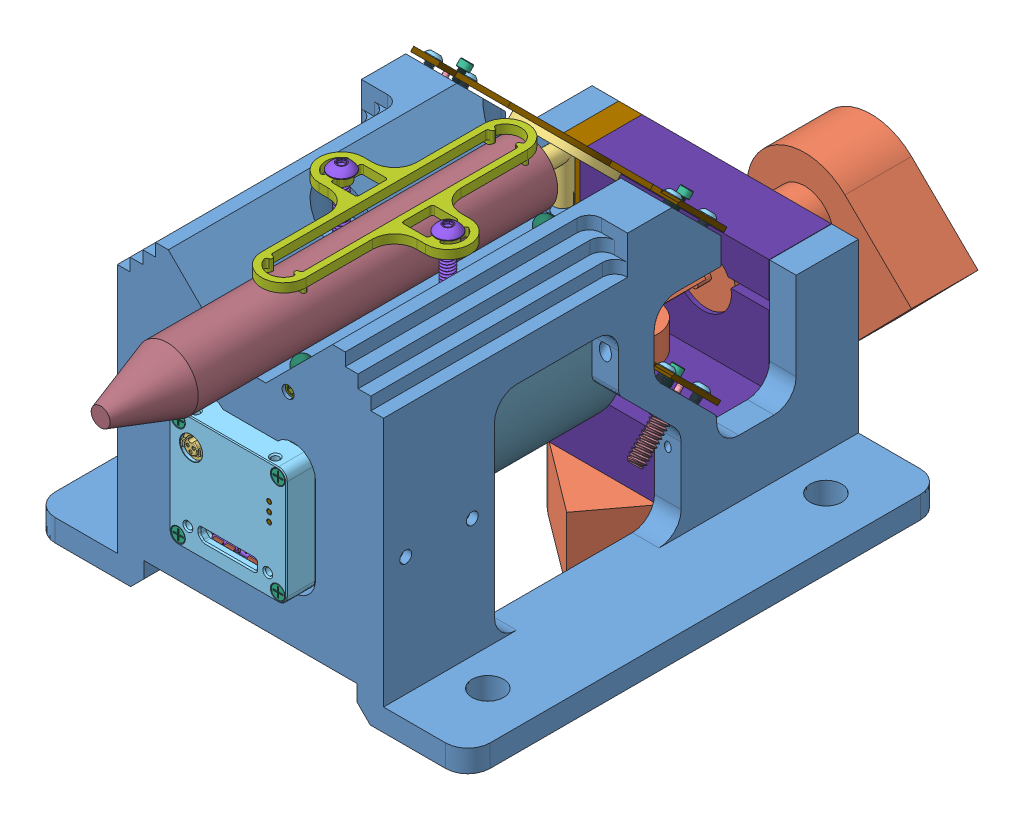
SolidWorks assembly cam_assem, configuration Default. Lengths in mm.
Overall size (98 162.28 212.1).
84 component instances, 45 part files, 76 mates.
Components (placement in the parent):
- cam_holder-1: cam_holder [Default] at origin size (98 71.23 107)
- STP-MQ-(MQ022xG-CM)-ASSM-1: STP-MQ-(MQ022xG-CM)-ASSM [Default] at (0 -13.2 7.5) x (-1 0 0) z (0 0 -1) size (26.4 26.4 30.19)
  - STP-MQ-(MQ022xG-CM)-ASSM.stp-1: STP-MQ-(MQ022xG-CM)-ASSM.stp [Default] at origin size (26.4 26.4 30.19)
    - SUBASSM-MQ-FRONT.stp-1: SUBASSM-MQ-FRONT.stp [Default] x (0 -1 0) z (0 0 1) size (26.4 26.4 14.6)
      - MECH-MQ-FRONT.stp-1: MECH-MQ-FRONT.stp [Default] at (0 0 7.5) x (1 0 0) z (0 0 -1) size (26.4 26.4 7.5)
      - MECH-MQ-CS-C.stp-1: MECH-MQ-CS-C.stp [Default] at (0 0 0.5) x (1 0 0) z (0 0 -1) size (26.4 26.4 5.5)
      - SROB-M2x14-CUST.stp-1: SROB-M2x14-CUST.stp [Default] at (-11.25 11.25 -7.1) size (3 3 14.55)
      - SROB-M2x14-CUST.stp-2: SROB-M2x14-CUST.stp [Default] at (11.25 -11.25 -7.1) size (3 3 14.55)
      - SROB-M2x14-CUST.stp-3: SROB-M2x14-CUST.stp [Default] at (11.25 11.25 -7.1) size (3 3 14.55)
      - SROB-M2x14-CUST.stp-4: SROB-M2x14-CUST.stp [Default] at (-11.25 -11.25 -7.1) size (3 3 14.55)
    - SUBASSM-MQ-REAR.stp-1: SUBASSM-MQ-REAR.stp [Default] at (0 0 -22.584) x (-1 0 0) z (0 0 1) size (26.4 26.4 10.6)
      - MECH-MQ-REAR.stp-1: MECH-MQ-REAR.stp [Default] at (0 0 6.5) x (-1 0 0) z (0 0 -1) size (26.4 26.4 6.5)
      - SROB-M2x10-CUST .stp-1: SROB-M2x10-CUST .stp [Default] at (-11.25 11.25 10.6) x (1 0 0) z (0 0 -1) size (3 3 10.55)
      - SROB-M2x10-CUST .stp-2: SROB-M2x10-CUST .stp [Default] at (11.25 11.25 10.6) x (1 0 0) z (0 0 -1) size (3 3 10.55)
      - SROB-M2x10-CUST .stp-3: SROB-M2x10-CUST .stp [Default] at (11.25 -11.25 10.6) x (1 0 0) z (0 0 -1) size (3 3 10.55)
      - SROB-M2x10-CUST .stp-4: SROB-M2x10-CUST .stp [Default] at (-11.25 -11.25 10.6) x (1 0 0) z (0 0 -1) size (3 3 10.55)
      - MECH-MQ-THERMAL-PAD.stp-1: MECH-MQ-THERMAL-PAD.stp [Default] at (-10.5 5.45 4.8) x (0.961741 -0.273959 0) z (0 0 -1) size (20.28 8 0.5)
      - MECH-EMI-GSKT-1.3X2.3X11.stp-1: MECH-EMI-GSKT-1.3X2.3X11.stp [Default] at (0 9.9495 3.45) size (11 1.2 3)
      - MECH-EMI-GSKT-1.3X2.3X11.stp-2: MECH-EMI-GSKT-1.3X2.3X11.stp [Default] at (0 7.0505 3.45) size (11 1.2 3)
      - MECH-LIGHTPIPE-1.63X4.14.stp-1: MECH-LIGHTPIPE-1.63X4.14.stp [Default] at (9.3 -3.5 4.1492) x (-1 0 0) z (0 -1 0) size (1.63 4.14 1.63)
      - MECH-LIGHTPIPE-1.63X4.14.stp-2: MECH-LIGHTPIPE-1.63X4.14.stp [Default] at (9.3 -1.5 4.1492) x (-1 0 0) z (0 -1 0) size (1.63 4.14 1.63)
      - MECH-LIGHTPIPE-1.63X4.14.stp-3: MECH-LIGHTPIPE-1.63X4.14.stp [Default] at (9.3 -5.5 4.1492) x (-1 0 0) z (0 -1 0) size (1.63 4.14 1.63)
    - SUBASSM-MQ-MID-022-CM.stp-1: SUBASSM-MQ-MID-022-CM.stp [Default] at (0 0 -4.5) x (-1 0 0) z (0 0 -1) size (26.4 26.4 11.68)
      - MECH-MQ-MID-022-CM-REV2.stp-1: MECH-MQ-MID-022-CM-REV2.stp [Default] at origin size (26.4 26.4 11.59)
      - MECH-O-RING-22X1-VI370.stp-1: MECH-O-RING-22X1-VI370.stp [Default] at (0 0 1.3) x (1 0 0) z (0 1 0) size (24 1 24)
      - FLT-BK7-AR2X-D25.stp-1: FLT-BK7-AR2X-D25.stp [Default] at (0 0 -0.1) size (25 25 1.1)
      - MECH-MX022xG-CM-GSKT.stp-1: MECH-MX022xG-CM-GSKT.stp [Default] at (0 0 3.364) x (0 -1 0) z (0 0 1) size (12.2 17.4 1.27)
    - MQ022xG-CM-PCA-LW_MODEL.stp-1: MQ022xG-CM-PCA-LW_MODEL.stp [Default] at (0 0 -16.486) x (-1 0 0) z (0 0 -1) size (25.43 25.43 13.85)
      - CMV2000.stp-1: CMV2000.stp [Default] at (-0.0259 -0.5261 -1.002) x (-1 0 0) z (0 0 -1) size (18.65 13.5 6.65)
        - ANDON-96UPGA-Socket.stp-1: ANDON-96UPGA-Socket.stp [Default] at origin size (15.9 10.8 3.23)
        - CMV2000_Package.stp-1: CMV2000_Package.stp [Default] at (0 0 3.29) x (-1 0 0) z (0 0 1) size (18.65 13.5 5.45)
        - CMV2000_Glass.stp-1: CMV2000_Glass.stp [Default] at (0 0 6.1) size (18.06 12.95 0.55)
      - MQ022xG-CM-PCA-LW_MODEL-0.stp-1: MQ022xG-CM-PCA-LW_MODEL-0.stp [Default] at origin size (0.25 1.57 4.1)
      - MQ022xG-CM-PCA-LW_MODEL-1.stp-1: MQ022xG-CM-PCA-LW_MODEL-1.stp [Default] at origin size (12.85 2.05 3.8)
      - MQ022xG-CM-PCA-LW_MODEL-2.stp-1: MQ022xG-CM-PCA-LW_MODEL-2.stp [Default] at origin size (25.43 25.43 1)
      - MQ022xG-CM-PCA-LW_MODEL-3.stp-1: MQ022xG-CM-PCA-LW_MODEL-3.stp [Default] at origin size (0.25 1.57 4.1)
      - MQ022xG-CM-PCA-LW_MODEL-4.stp-1: MQ022xG-CM-PCA-LW_MODEL-4.stp [Default] at origin size (5 5 8.1)
      - MQ022xG-CM-PCA-LW_MODEL-5.stp-1: MQ022xG-CM-PCA-LW_MODEL-5.stp [Default] at origin size (0.25 1.57 4.1)
      - MQ022xG-CM-PCA-LW_MODEL-6.stp-1: MQ022xG-CM-PCA-LW_MODEL-6.stp [Default] at origin size (0.25 1.57 4.1)
      - MQ022xG-CM-PCA-LW_MODEL-7.stp-1: MQ022xG-CM-PCA-LW_MODEL-7.stp [Default] at origin size (0.25 1.57 4.1)
      - MQ022xG-CM-PCA-LW_MODEL-8.stp-1: MQ022xG-CM-PCA-LW_MODEL-8.stp [Default] at origin size (0.25 1.57 4.1)
      - MQ022xG-CM-PCA-LW_MODEL-9.stp-1: MQ022xG-CM-PCA-LW_MODEL-9.stp [Default] at origin size (0.25 1.57 4.1)
      - MQ022xG-CM-PCA-LW_MODEL-10.stp-1: MQ022xG-CM-PCA-LW_MODEL-10.stp [Default] at origin size (0.25 1.57 4.1)
      - MQ022xG-CM-PCA-LW_MODEL-11.stp-1: MQ022xG-CM-PCA-LW_MODEL-11.stp [Default] at origin size (0.25 1.57 4.1)
      - MQ022xG-CM-PCA-LW_MODEL-12.stp-1: MQ022xG-CM-PCA-LW_MODEL-12.stp [Default] at origin size (13.8 3 5.6)
      - MQ022xG-CM-PCA-LW_MODEL-13.stp-1: MQ022xG-CM-PCA-LW_MODEL-13.stp [Default] at origin size (0.25 1.57 4.1)
- laser-1: laser [Default] at (0 18.5208 -37.2385) x (0 -1 0) z (0 0 1) size (14 14 96)
- lens-1: lens [Default] at (0 -13.2 -42) x (0 1 0) z (0 0 1) size (33.5 33.5 46.7)
- 1598K25_Hardened Bearing-Quality 440C Stainless Steel Ball-1: 1598K25_Hardened Bearing-Quality 440C Stainless Steel Ball [1598K25] at (-6.6608 12.5671 20) x (0.595435 0.636273 0.490525) z (-0.571952 -0.093063 0.814991) size (4 4 4)
- 92695A729_Alloy Steel Cone-Point Set Screws-1: 92695A729_Alloy Steel Cone-Point Set Screws [92695A729] at (-8.4853 10.8376 24.4029) x (0.913011 -0.407935 0) z (0 0 1) size (4.05 3.54 3.43)
- 1598K25_Hardened Bearing-Quality 440C Stainless Steel Ball-2: 1598K25_Hardened Bearing-Quality 440C Stainless Steel Ball [1598K25] at (-6.364 12.1569 -35) x (0.756378 0.1991 0.623098) z (-0.446406 -0.539153 0.714168) size (4 4 4)
- 1598K25_Hardened Bearing-Quality 440C Stainless Steel Ball-4: 1598K25_Hardened Bearing-Quality 440C Stainless Steel Ball [1598K25] at (6.364 12.1569 -35) x (0.295652 0.723786 0.623477) z (-0.259043 -0.567459 0.781593) size (4 4 4)
- galvo_block-1: galvo_block [Default] at (-18.725 -27.865 -82) x (0 -1 0) z (1 0 0) size (39.65 34.73 42.65)
- D_holder-1: D_holder [Default] at (0 -12.8464 -45.6926) x (1 0 0) z (0 -0.707107 0.707107) size (60 22 1)
- D-1: D [Default] at (0 -13.2 -45.339) x (1 0 0) z (0 -0.707107 0.707107) size (20 121.63 78.36)
- glavo-1: glavo [Default] at (0 -58.6069 -60.255) x (0.599182 0 -0.800613) z (0.800613 0 0.599182) size (26 51 34)
- D_holder-2: D_holder [Default] at (0 20.2886 -47.1068) x (1 0 0) z (0 -0.707107 0.707107) size (60 22 1)
- mirror-1: mirror [Default] at (0 18.5208 -45.339) x (-1 0 0) z (0 0.707107 -0.707107) size (20 121.63 78.36)
- 3126A21_Slotted Long-Nose Steel Spring Plunger-1: 3126A21_Slotted Long-Nose Steel Spring Plunger [3126A21] at (27 -19.2382 -39.3008) x (0.917455 -0.281315 -0.281315) z (0.397839 0.648739 0.648739) size (3.52 15.42 3.68)
- 92949A319_18-8 Stainless Steel Button Head Hex Drive Screw-1: 92949A319_18-8 Stainless Steel Button Head Hex Drive Screw [92949A319] at (27 -10.9061 -39.8548) x (-0.780279 -0.442247 -0.442247) z (0 0.707107 -0.707107) size (3.28 3.28 7.4)
- 92196A051_18-8 Stainless Steel Socket Head Screw-1: 92196A051_18-8 Stainless Steel Socket Head Screw [92196A051] at (24.75 -13.1743 -45.3647) x (-0.756852 -0.462156 -0.462156) z (0 0.707107 -0.707107) size (2.44 2.44 4.07)
- 92949A319_18-8 Stainless Steel Button Head Hex Drive Screw-2: 92949A319_18-8 Stainless Steel Button Head Hex Drive Screw [92949A319] at (27 -18.6842 -47.633) x (-0.793626 -0.430208 -0.430208) z (0 0.707107 -0.707107) size (3.28 3.28 7.4)
- 92949A319_18-8 Stainless Steel Button Head Hex Drive Screw-3: 92949A319_18-8 Stainless Steel Button Head Hex Drive Screw [92949A319] at (-27 -10.9061 -39.8548) x (-0.831896 -0.392395 -0.392395) z (0 0.707107 -0.707107) size (3.28 3.28 7.4)
- 92949A319_18-8 Stainless Steel Button Head Hex Drive Screw-4: 92949A319_18-8 Stainless Steel Button Head Hex Drive Screw [92949A319] at (-27 -18.6842 -47.633) x (-0.88833 -0.324707 -0.324707) z (0 0.707107 -0.707107) size (3.28 3.28 7.4)
- 92196A051_18-8 Stainless Steel Socket Head Screw-2: 92196A051_18-8 Stainless Steel Socket Head Screw [92196A051] at (-24.75 -13.1164 -45.4227) x (-0.770813 -0.45047 -0.45047) z (0 0.707107 -0.707107) size (2.44 2.44 4.07)
- 3126A21_Slotted Long-Nose Steel Spring Plunger-3: 3126A21_Slotted Long-Nose Steel Spring Plunger [3126A21] at (-27 -19.4685 -39.0705) x (0.908634 -0.295283 -0.295283) z (0.417593 0.642502 0.642502) size (3.52 15.42 3.68)
- 3126A21_Slotted Long-Nose Steel Spring Plunger-5: 3126A21_Slotted Long-Nose Steel Spring Plunger [3126A21] at (-27 13.9393 -40.5359) x (0.687618 -0.513411 -0.513411) z (0.726072 0.48622 0.48622) size (3.52 15.42 3.68)
- 92949A319_18-8 Stainless Steel Button Head Hex Drive Screw-7: 92949A319_18-8 Stainless Steel Button Head Hex Drive Screw [92949A319] at (27 22.229 -41.269) x (-0.793626 -0.430208 -0.430208) z (0 0.707107 -0.707107) size (3.28 3.28 7.4)
- 92949A319_18-8 Stainless Steel Button Head Hex Drive Screw-10: 92949A319_18-8 Stainless Steel Button Head Hex Drive Screw [92949A319] at (27 14.4508 -49.0472) x (-0.806602 -0.417967 -0.417967) z (0 0.707107 -0.707107) size (3.28 3.28 7.4)
- 92949A319_18-8 Stainless Steel Button Head Hex Drive Screw-11: 92949A319_18-8 Stainless Steel Button Head Hex Drive Screw [92949A319] at (-27 22.229 -41.269) x (-0.843706 -0.379579 -0.379579) z (0 0.707107 -0.707107) size (3.28 3.28 7.4)
- 92949A319_18-8 Stainless Steel Button Head Hex Drive Screw-12: 92949A319_18-8 Stainless Steel Button Head Hex Drive Screw [92949A319] at (-27 14.4508 -49.0472) x (-0.898056 -0.311043 -0.311043) z (0 0.707107 -0.707107) size (3.28 3.28 7.4)
- 92196A051_18-8 Stainless Steel Socket Head Screw-4: 92196A051_18-8 Stainless Steel Socket Head Screw [92196A051] at (24.75 20.4716 -47.2898) x (-0.770813 -0.45047 -0.45047) z (0 0.707107 -0.707107) size (2.44 2.44 4.07)
- 92196A051_18-8 Stainless Steel Socket Head Screw-6: 92196A051_18-8 Stainless Steel Socket Head Screw [92196A051] at (-24.75 20.4716 -47.2898) x (-0.784414 -0.438574 -0.438574) z (0 0.707107 -0.707107) size (2.44 2.44 4.07)
- 3126A21_Slotted Long-Nose Steel Spring Plunger-7: 3126A21_Slotted Long-Nose Steel Spring Plunger [3126A21] at (0 -34.7439 20) size (3.52 15.42 3.68)
- 3126A21_Slotted Long-Nose Steel Spring Plunger-8: 3126A21_Slotted Long-Nose Steel Spring Plunger [3126A21] at (0 -34.7439 5) x (0.982082 0 -0.188455) z (0.188455 0 0.982082) size (3.52 15.42 3.68)
- 3126A21_Slotted Long-Nose Steel Spring Plunger-10: 3126A21_Slotted Long-Nose Steel Spring Plunger [3126A21] at (21.5439 -13.2 20) x (0 0.999599 -0.02833) z (0 0.02833 0.999599) size (3.52 15.42 3.68)
- 3126A21_Slotted Long-Nose Steel Spring Plunger-12: 3126A21_Slotted Long-Nose Steel Spring Plunger [3126A21] at (21.5439 -13.2 5) x (0 0.991446 0.130517) z (0 -0.130517 0.991446) size (3.52 15.42 3.68)
- clamp-1: clamp [Default] at (0 27.583 -7.5) x (0 0 -1) z (-1 0 0) size (60 3 34)
- 92949A113_18-8 Stainless Steel Button Head Hex Drive Screw-1: 92949A113_18-8 Stainless Steel Button Head Hex Drive Screw [92949A113] at (12 18.8073 -7.5) x (-0.837169 0 -0.546944) z (0 1 0) size (5.41 5.41 20.93)
- 92949A113_18-8 Stainless Steel Button Head Hex Drive Screw-2: 92949A113_18-8 Stainless Steel Button Head Hex Drive Screw [92949A113] at (-12 18.8073 -7.5) x (-0.925243 0 -0.379375) z (0 1 0) size (5.41 5.41 20.93)
- 1598K25_Hardened Bearing-Quality 440C Stainless Steel Ball-6: 1598K25_Hardened Bearing-Quality 440C Stainless Steel Ball [1598K25] at (6.7083 12.5196 20) x (-0.036454 0.98158 0.187543) z (-0.758508 -0.149364 0.634315) size (4 4 4)
- 92695A729_Alloy Steel Cone-Point Set Screws-2: 92695A729_Alloy Steel Cone-Point Set Screws [92695A729] at (8.4729 10.7426 24.2676) x (0.992207 -0.1246 0) z (0 0 1) size (4.05 3.54 3.43)
- glavo-2: glavo [Default] at (9 -13.2 -105.8802) x (0.700486 0.713666 0) z (0.713666 -0.700486 0) size (26 51 34)
- spacer-1: spacer [Default] at (-24.005 -27.865 -82) x (0 -1 0) z (1 0 0) size (39.65 34.73 5.28)
Mates (geometry in assembly coordinates):
- Coincident2: coincident anti-aligned: plane of STP-MQ-(MQ022xG-CM)-ASSM-1 through (0 -13.2 7.5) normal (-1 0 0)
- Concentric2: concentric: cylinder of cam_holder-1 through (-8.4853 10.7426 20) axis (0.707107 0.707107 0) radius 2; sphere of 1598K25_Hardened Bearing-Quality 440C Stainless Steel Ball-1
- Concentric5: concentric aligned: cylinder of STP-MQ-(MQ022xG-CM)-ASSM-1/STP-MQ-(MQ022xG-CM)-ASSM.stp-1/SUBASSM-MQ-FRONT.stp-1/MECH-MQ-FRONT.stp-1 through (0 -13.2 6.5) axis (0 0 -1) radius 12.2703; cylinder of lens-1 through (0 -13.2 4.7) axis (0 0 -1) radius 12.65
- Coincident3: coincident anti-aligned: plane of STP-MQ-(MQ022xG-CM)-ASSM-1/STP-MQ-(MQ022xG-CM)-ASSM.stp-1/SUBASSM-MQ-FRONT.stp-1/MECH-MQ-FRONT.stp-1 through (-13.2 0 0) normal (0 0 -1); plane of lens-1 through (0 -13.2 0) normal (0 0 1)
- Coincident4: coincident anti-aligned: plane of cam_holder-1 through (-13.2 0 25) normal (0 -1 0); plane of STP-MQ-(MQ022xG-CM)-ASSM-1/STP-MQ-(MQ022xG-CM)-ASSM.stp-1/SUBASSM-MQ-MID-022-CM.stp-1/MECH-MQ-MID-022-CM-REV2.stp-1 through (13.2 0 23.584) normal (0 1 0)
- Parallel1: parallel aligned: plane of lens-1 through (0 -13.2 -42) normal (0 1 0)
- Coincident7: coincident aligned: plane of lens-1 through (0 -13.2 -42) normal (0 1 0); plane of galvo_block-1 through (-18.725 -13.2 -82) normal (0 1 0)
- Coincident8: coincident anti-aligned: plane of cam_holder-1 through (0 0 0) normal (0 0 -1); plane of lens-1 through (0 -13.2 0) normal (0 0 1)
- Coincident9: coincident aligned: plane of lens-1 through (0 -13.2 -42) normal (-1 0 0); plane of galvo_block-1 through (0 -27.865 -82) normal (-1 0 0)
- Coincident10: coincident aligned: plane of cam_holder-1 through (0 0 -82) normal (0 0 -1); plane of galvo_block-1 through (23.925 -27.865 -82) normal (0 0 -1)
- Concentric6: concentric anti-aligned: cylinder of D_holder-1 through (0 -13.2 -45.339) axis (0 -0.707107 0.707107) radius 10; cylinder of D-1 through (0 -14.6142 -43.9248) axis (0 0.707107 -0.707107) radius 10
- Coincident12: coincident anti-aligned: plane of D_holder-1 through (0 -13.2 -45.339) normal (0 -0.707107 0.707107); plane of D-1 through (0 -13.2 -45.339) normal (0 0.707107 -0.707107)
- Coincident14: coincident aligned: plane of lens-1 through (0 -13.2 -42) normal (0 1 0); plane of D_holder-1 through (0 -13.2 -45.6926) normal (0 1 0)
- Coincident15: coincident anti-aligned: plane of lens-1 through (0 -13.2 -42) normal (-1 0 0); plane of D_holder-1 through (0 -12.8464 -45.6926) normal (1 0 0)
- Concentric7: concentric anti-aligned: cylinder of galvo_block-1 through (0 -70.515 -60.255) axis (0 1 0) radius 6.425; cylinder of glavo-1 through (0 -21.6069 -60.255) axis (0 -1 0) radius 6.5
- Concentric8: concentric aligned: cylinder of D_holder-2 through (0 19.935 -46.7533) axis (0 -0.707107 0.707107) radius 10; cylinder of mirror-1 through (0 19.935 -46.7533) axis (0 -0.707107 0.707107) radius 10
- Coincident16: coincident anti-aligned: plane of D_holder-2 through (0 19.935 -46.7533) normal (0 -0.707107 0.707107); plane of mirror-1 through (0 19.935 -46.7533) normal (0 0.707107 -0.707107)
- Concentric9: concentric aligned: cylinder of laser-1 through (0 18.5208 58.7615) axis (0 0 -1) radius 7; axis of mirror-1 through (0 18.5208 -25.339) axis (0 0 -1)
- Coincident17: coincident aligned: plane of laser-1 through (0 18.5208 -37.2385) normal (1 0 0)
- Parallel2: parallel anti-aligned: plane of laser-1 through (0 18.5208 -37.2385) normal (0 -1 0)
- Parallel3: parallel anti-aligned: plane of cam_holder-1 through (49 8 -57) normal (0 0.707107 -0.707107); plane of D_holder-2 through (0 19.5815 -46.3997) normal (0 -0.707107 0.707107)
- Coincident20: coincident aligned: plane of D_holder-2 through (0 20.2886 -47.1068) normal (1 0 0)
- Concentric10: concentric anti-aligned: cylinder of D-1 through (0 6.8 -45.339) axis (0 -1 0) radius 2; cylinder of mirror-1 through (0 8.5208 -45.339) axis (0 1 0) radius 2
- Concentric11: concentric aligned: cylinder of cam_holder-1 through (27 -14.5551 -43.984) axis (0 0.707107 -0.707107) radius 1.3526; cylinder of 3126A21_Slotted Long-Nose Steel Spring Plunger-1 through (27 -13.3382 -45.2008) axis (0 0.707107 -0.707107) radius 0.5715
- Concentric12: concentric aligned: cylinder of D_holder-1 through (27 -8.9574 -41.8035) axis (0 0.707107 -0.707107) radius 1.1303; cylinder of 92949A319_18-8 Stainless Steel Button Head Hex Drive Screw-1 through (27 -8.3647 -42.3962) axis (0 0.707107 -0.707107) radius 1.6383
- Coincident21: coincident anti-aligned: plane of D_holder-1 through (0 -12.8464 -45.6926) normal (0 0.707107 -0.707107); plane of 92949A319_18-8 Stainless Steel Button Head Hex Drive Screw-1 through (25.9754 -8.0534 -40.8996) normal (0 -0.707107 0.707107)
- Concentric13: concentric anti-aligned: cylinder of D_holder-1 through (24.75 -12.8464 -45.6926) axis (0 0.707107 -0.707107) radius 0.5956; cylinder of 92196A051_18-8 Stainless Steel Socket Head Screw-1 through (24.75 -14.5551 -43.984) axis (0 -0.707107 0.707107) radius 1.2192
- Concentric14: concentric aligned: cylinder of cam_holder-1 through (27 -10.666 -40.0949) axis (0 0.707107 -0.707107) radius 0.7556; cylinder of 92949A319_18-8 Stainless Steel Button Head Hex Drive Screw-1 through (27 -8.3647 -42.3962) axis (0 0.707107 -0.707107) radius 1.6383
- Coincident22: coincident anti-aligned: plane of cam_holder-1 through (49 -20.0563 -49.4853) normal (0 0.707107 -0.707107); plane of 92196A051_18-8 Stainless Steel Socket Head Screw-1 through (24.4076 -14.2747 -43.7036) normal (0 -0.707107 0.707107)
- Concentric15: concentric aligned: cylinder of D_holder-1 through (27 -16.7355 -49.5817) axis (0 0.707107 -0.707107) radius 1.1303; cylinder of 92949A319_18-8 Stainless Steel Button Head Hex Drive Screw-2 through (27 -16.1428 -50.1744) axis (0 0.707107 -0.707107) radius 1.6383
- Coincident23: coincident anti-aligned: plane of D_holder-1 through (0 -12.8464 -45.6926) normal (0 0.707107 -0.707107); plane of 92949A319_18-8 Stainless Steel Button Head Hex Drive Screw-2 through (26.0032 -15.8162 -48.6623) normal (0 -0.707107 0.707107)
- Concentric16: concentric aligned: cylinder of D_holder-1 through (-27 -8.9574 -41.8035) axis (0 0.707107 -0.707107) radius 1.1303; cylinder of 92949A319_18-8 Stainless Steel Button Head Hex Drive Screw-3 through (-27 -8.3647 -42.3962) axis (0 0.707107 -0.707107) radius 1.6383
- Coincident26: coincident anti-aligned: plane of D_holder-1 through (0 -12.8464 -45.6926) normal (0 0.707107 -0.707107); plane of 92949A319_18-8 Stainless Steel Button Head Hex Drive Screw-3 through (-27.9091 -7.9936 -40.8398) normal (0 -0.707107 0.707107)
- Coincident27: coincident anti-aligned: plane of D_holder-1 through (0 -12.8464 -45.6926) normal (0 0.707107 -0.707107); plane of 92949A319_18-8 Stainless Steel Button Head Hex Drive Screw-4 through (-27.7523 -15.7064 -48.5526) normal (0 -0.707107 0.707107)
- Concentric17: concentric aligned: cylinder of D_holder-1 through (-27 -16.7355 -49.5817) axis (0 0.707107 -0.707107) radius 1.1303; cylinder of 92949A319_18-8 Stainless Steel Button Head Hex Drive Screw-4 through (-27 -16.1428 -50.1744) axis (0 0.707107 -0.707107) radius 1.6383
- Concentric18: concentric anti-aligned: cylinder of D_holder-1 through (-24.75 -12.8464 -45.6926) axis (0 0.707107 -0.707107) radius 0.5956; cylinder of 92196A051_18-8 Stainless Steel Socket Head Screw-2 through (-24.75 -14.4971 -44.0419) axis (0 -0.707107 0.707107) radius 1.2192
- Concentric19: concentric aligned: cylinder of cam_holder-1 through (-27 -14.5551 -43.984) axis (0 0.707107 -0.707107) radius 1.3526; cylinder of 3126A21_Slotted Long-Nose Steel Spring Plunger-3 through (-27 -13.5685 -44.9705) axis (0 0.707107 -0.707107) radius 0.5715
- Concentric20: concentric aligned: cylinder of cam_holder-1 through (-27 19.2017 -45.7983) axis (0 0.707107 -0.707107) radius 1.3526; cylinder of 3126A21_Slotted Long-Nose Steel Spring Plunger-5 through (-27 19.8394 -46.4359) axis (0 0.707107 -0.707107) radius 0.5715
- Concentric22: concentric aligned: cylinder of D_holder-2 through (27 24.1777 -43.2177) axis (0 0.707107 -0.707107) radius 1.1303; cylinder of 92949A319_18-8 Stainless Steel Button Head Hex Drive Screw-7 through (27 24.7704 -43.8104) axis (0 0.707107 -0.707107) radius 1.6383
- Coincident29: coincident anti-aligned: plane of D_holder-2 through (0 20.2886 -47.1068) normal (0 0.707107 -0.707107); plane of 92949A319_18-8 Stainless Steel Button Head Hex Drive Screw-7 through (26.0032 25.097 -42.2983) normal (0 -0.707107 0.707107)
- Concentric24: concentric aligned: cylinder of D_holder-2 through (27 16.3995 -50.9959) axis (0 0.707107 -0.707107) radius 1.1303; cylinder of 92949A319_18-8 Stainless Steel Button Head Hex Drive Screw-10 through (27 16.9922 -51.5886) axis (0 0.707107 -0.707107) radius 1.6383
- Coincident31: coincident anti-aligned: plane of D_holder-2 through (0 20.2886 -47.1068) normal (0 0.707107 -0.707107); plane of 92949A319_18-8 Stainless Steel Button Head Hex Drive Screw-10 through (26.0316 17.3339 -50.0615) normal (0 -0.707107 0.707107)
- Coincident32: coincident anti-aligned: plane of D_holder-2 through (0 20.2886 -47.1068) normal (0 0.707107 -0.707107); plane of 92949A319_18-8 Stainless Steel Button Head Hex Drive Screw-11 through (-27.8794 25.1551 -42.2403) normal (0 -0.707107 0.707107)
- Concentric25: concentric aligned: cylinder of D_holder-2 through (-27 24.1777 -43.2177) axis (0 0.707107 -0.707107) radius 1.1303; cylinder of 92949A319_18-8 Stainless Steel Button Head Hex Drive Screw-11 through (-27 24.7704 -43.8104) axis (0 0.707107 -0.707107) radius 1.6383
- Coincident33: coincident anti-aligned: plane of D_holder-2 through (0 20.2886 -47.1068) normal (0 0.707107 -0.707107); plane of 92949A319_18-8 Stainless Steel Button Head Hex Drive Screw-12 through (-27.7207 17.4399 -49.9555) normal (0 -0.707107 0.707107)
- Concentric26: concentric aligned: cylinder of D_holder-2 through (-27 16.3995 -50.9959) axis (0 0.707107 -0.707107) radius 1.1303; cylinder of 92949A319_18-8 Stainless Steel Button Head Hex Drive Screw-12 through (-27 16.9922 -51.5886) axis (0 0.707107 -0.707107) radius 1.6383
- Concentric27: concentric anti-aligned: cylinder of D_holder-2 through (24.75 20.2886 -47.1068) axis (0 0.707107 -0.707107) radius 0.5956; cylinder of 92196A051_18-8 Stainless Steel Socket Head Screw-4 through (24.75 19.0909 -45.9091) axis (0 -0.707107 0.707107) radius 1.2192
- Coincident36: coincident anti-aligned: plane of cam_holder-1 through (49 8 -57) normal (0 0.707107 -0.707107); plane of 92196A051_18-8 Stainless Steel Socket Head Screw-4 through (24.4163 19.3764 -45.6236) normal (0 -0.707107 0.707107)
- Concentric28: concentric anti-aligned: cylinder of D_holder-2 through (-24.75 20.2886 -47.1068) axis (0 0.707107 -0.707107) radius 0.5956; cylinder of 92196A051_18-8 Stainless Steel Socket Head Screw-6 through (-24.75 19.0909 -45.9091) axis (0 -0.707107 0.707107) radius 1.2192
- Coincident37: coincident anti-aligned: plane of cam_holder-1 through (49 8 -57) normal (0 0.707107 -0.707107); plane of 92196A051_18-8 Stainless Steel Socket Head Screw-6 through (-25.0749 19.3815 -45.6185) normal (0 -0.707107 0.707107)
- Concentric29: concentric anti-aligned: cylinder of cam_holder-1 through (0 -38.4 20) axis (0 -1 0) radius 1.3526; line of 3126A21_Slotted Long-Nose Steel Spring Plunger-7 through (0 -27.3144 20) axis (0 1 0)
- Tangent6: tangent anti-aligned: plane of STP-MQ-(MQ022xG-CM)-ASSM-1/STP-MQ-(MQ022xG-CM)-ASSM.stp-1/SUBASSM-MQ-MID-022-CM.stp-1/MECH-MQ-MID-022-CM-REV2.stp-1 through (-13.2 -26.4 23.584) normal (0 -1 0); sphere of 3126A21_Slotted Long-Nose Steel Spring Plunger-7
- Concentric30: concentric anti-aligned: cylinder of cam_holder-1 through (0 -38.4 5) axis (0 -1 0) radius 1.3526; line of 3126A21_Slotted Long-Nose Steel Spring Plunger-8 through (0 -27.3144 5) axis (0 1 0)
- Tangent7: tangent anti-aligned: plane of STP-MQ-(MQ022xG-CM)-ASSM-1/STP-MQ-(MQ022xG-CM)-ASSM.stp-1/SUBASSM-MQ-MID-022-CM.stp-1/MECH-MQ-MID-022-CM-REV2.stp-1 through (-13.2 -26.4 23.584) normal (0 -1 0); sphere of 3126A21_Slotted Long-Nose Steel Spring Plunger-8
- Concentric31: concentric anti-aligned: cylinder of cam_holder-1 through (30 -13.2 20) axis (1 0 0) radius 1.3526; line of 3126A21_Slotted Long-Nose Steel Spring Plunger-10 through (14.1144 -13.2 20) axis (-1 0 0)
- Tangent9: tangent anti-aligned: plane of STP-MQ-(MQ022xG-CM)-ASSM-1/STP-MQ-(MQ022xG-CM)-ASSM.stp-1/SUBASSM-MQ-REAR.stp-1/MECH-MQ-REAR.stp-1 through (13.2 -26.4 30.084) normal (1 0 0); sphere of 3126A21_Slotted Long-Nose Steel Spring Plunger-10
- Concentric32: concentric anti-aligned: cylinder of cam_holder-1 through (30 -13.2 5) axis (1 0 0) radius 1.3526; line of 3126A21_Slotted Long-Nose Steel Spring Plunger-12 through (14.1144 -13.2 5) axis (-1 0 0)
- Tangent10: tangent anti-aligned: plane of STP-MQ-(MQ022xG-CM)-ASSM-1/STP-MQ-(MQ022xG-CM)-ASSM.stp-1/SUBASSM-MQ-REAR.stp-1/MECH-MQ-REAR.stp-1 through (13.2 -26.4 30.084) normal (1 0 0); sphere of 3126A21_Slotted Long-Nose Steel Spring Plunger-12
- Concentric33: concentric aligned: cylinder of cam_holder-1 through (-12 15 -7.5) axis (0 1 0) radius 1.1303; line of clamp-1 through (-12 25.583 -7.5) axis (0 1 0)
- Parallel4: parallel aligned: plane of cam_holder-1 through (-30 -40 25) normal (-1 0 0); plane of clamp-1 through (-5 25.583 17.5) normal (-1 0 0)
- Tangent14: tangent: cylinder of laser-1 through (0 18.5208 58.7615) axis (0 0 -1) radius 7; circle of clamp-1
- Concentric36: concentric aligned: cylinder of clamp-1 through (12 27.583 -7.5) axis (0 1 0) radius 1.4732; cylinder of 92949A113_18-8 Stainless Steel Button Head Hex Drive Screw-1 through (12 29.0816 -7.5) axis (0 1 0) radius 2.7051
- Coincident40: coincident anti-aligned: plane of clamp-1 through (0 27.583 17.5) normal (0 1 0); plane of 92949A113_18-8 Stainless Steel Button Head Hex Drive Screw-1 through (10.5205 27.583 -5.2354) normal (0 -1 0)
- Concentric37: concentric aligned: cylinder of clamp-1 through (-12 27.583 -7.5) axis (0 1 0) radius 1.4732; cylinder of 92949A113_18-8 Stainless Steel Button Head Hex Drive Screw-2 through (-12 29.0816 -7.5) axis (0 1 0) radius 2.7051
- Coincident41: coincident anti-aligned: plane of clamp-1 through (0 27.583 17.5) normal (0 1 0); plane of 92949A113_18-8 Stainless Steel Button Head Hex Drive Screw-2 through (-13.0262 27.583 -4.9971) normal (0 -1 0)
- Concentric38: concentric: cylinder of cam_holder-1 through (-7.7782 10.7426 -35) axis (0.707107 0.707107 0) radius 2; sphere of 1598K25_Hardened Bearing-Quality 440C Stainless Steel Ball-2
- Tangent16: tangent anti-aligned: plane of cam_holder-1 through (-7.7782 10.7426 -35) normal (0.707107 0.707107 0); sphere of 1598K25_Hardened Bearing-Quality 440C Stainless Steel Ball-2
- Concentric39: concentric: cylinder of cam_holder-1 through (7.7782 10.7426 -35) axis (-0.707107 0.707107 0) radius 2; sphere of 1598K25_Hardened Bearing-Quality 440C Stainless Steel Ball-4
- Tangent18: tangent anti-aligned: plane of cam_holder-1 through (7.7782 10.7426 -35) normal (-0.707107 0.707107 0); sphere of 1598K25_Hardened Bearing-Quality 440C Stainless Steel Ball-4
- Concentric41: concentric: cylinder of cam_holder-1 through (8.4853 10.7426 20) axis (-0.707107 0.707107 0) radius 2; sphere of 1598K25_Hardened Bearing-Quality 440C Stainless Steel Ball-6
- Tangent19: tangent aligned: cylinder of cam_holder-1 through (8.4853 10.7426 25) axis (0 0 1) radius 1.3526; face of 92695A729_Alloy Steel Cone-Point Set Screws-2
- Tangent20: tangent anti-aligned: cylinder of laser-1 through (0 18.5208 58.7615) axis (0 0 -1) radius 7; sphere of 1598K25_Hardened Bearing-Quality 440C Stainless Steel Ball-4
- Concentric42: concentric anti-aligned: cylinder of galvo_block-1 through (9 -13.2 -110.65) axis (0 0 1) radius 6.425; cylinder of glavo-2 through (9 -13.2 -68.8802) axis (0 0 -1) radius 6.5
- Coincident42: coincident: plane of galvo_block-1 through (23.925 -27.865 -82) normal (0 0 -1); plane of spacer-1 through (18.645 -27.865 -82) normal (0 0 -1)
- Coincident43: coincident: plane of galvo_block-1 through (-18.725 -27.865 -82) normal (-1 0 0); plane of spacer-1 through (-18.725 8.5536 -47.27) normal (1 0 0)
- Coincident44: coincident aligned: plane of galvo_block-1 through (23.925 -41.865 -82) normal (0 -1 0); plane of spacer-1 through (18.645 -41.865 -82) normal (0 -1 0)
